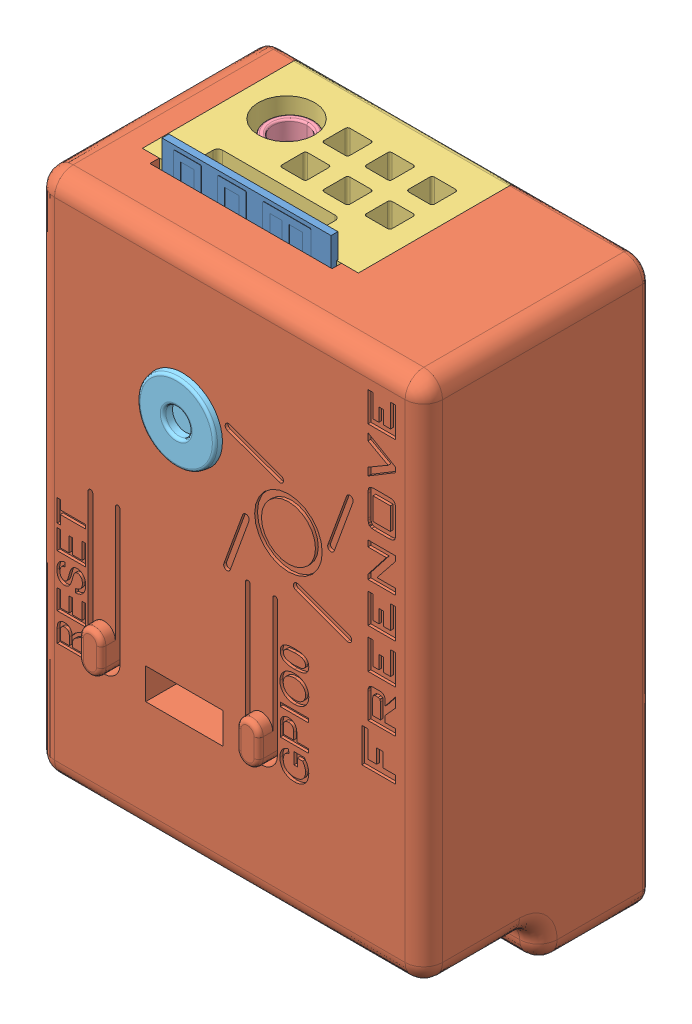
SolidWorks assembly FNK0102_Assembly_Has_Battery, configuration 默认. Lengths in mm.
Overall size (41.34 62.5 31.21).
6 component instances, 6 part files, 18 mates.
Components (placement in the parent):
- CB8201_20250427-1: CB8201_20250427 [默认] at (-3.6296 -20.6055 14.3314) x (1 0 0) z (0 0 1) size (27.94 57.2 13.09)
- FNK0102_Part1_v1.2-1: FNK0102_Part1_v1.2 [一体按键0.00间距] at (-3.8296 -20.4055 14.5) size (41.34 59.9 25.5)
- FNK0102_Part2_v1.2-1: FNK0102_Part2_v1.2 [0.0间距] at (-3.8296 30.3945 0) size (38.84 59.9 16.8)
- CB10201-1: CB10201 [默认] at (17.1633 5.4788 -53.4541) size (27.94 53.02 18.11)
- Camera_OV3660-1: Camera_OV3660 [默认] at (10.5364 16.4245 16.8) size (13.1 21.9 8.2)
- Battery_752035-1: Battery_752035 [默认] at (33.8104 2.3695 16.6198) x (0 1 0) z (-1 0 0) size (38 20 7.7)
Mates (geometry in assembly coordinates):
- 重合1: coincident: plane of assembly through (0 0 0) normal (0 0 1); plane of CB10201-1 through (-3.6296 -20.6055 0) normal (0 0 -1); plane of assembly
- 平行14: parallel: plane of assembly; plane of assembly; plane of FNK0102_Part1_v1.2-1 through (-4.0296 -20.4055 16.2) normal (1 0 0); plane of CB10201-1 through (-3.6296 30.1945 0) normal (-1 0 0)
- 重合30: coincident: plane of assembly; plane of assembly; plane of FNK0102_Part1_v1.2-1 through (-3.8296 -20.4055 -0.6) normal (0 0 -1); plane of FNK0102_Part2_v1.2-1 through (-3.8296 30.3945 -0.6) normal (0 0 1)
- 重合31: coincident: plane of assembly; plane of assembly; plane of FNK0102_Part1_v1.2-1 through (-3.8296 -26.1055 49.5331) normal (0 -1 0); plane of FNK0102_Part2_v1.2-1 through (10.1404 -26.1055 -0.6) normal (0 -1 0)
- 重合32: coincident: plane of assembly; plane of assembly; plane of FNK0102_Part1_v1.2-1 through (10.1404 -24.6055 -0.6) normal (1 0 0); plane of FNK0102_Part2_v1.2-1 through (10.1404 -24.6055 -0.6) normal (-1 0 0)
- 重合38: coincident: plane of assembly; plane of assembly; plane of CB8201_20250427-1 through (-3.6448 -20.8607 10.1) normal (0 0 -1); plane of CB10201-1 through (-1.0896 -19.3355 10.1) normal (0 0 1)
- 重合39: coincident: plane of assembly; plane of assembly; plane of CB8201_20250427-1 through (-3.4648 -20.6055 12.8952) normal (0 -1 0); plane of CB10201-1 through (-3.6296 -20.6055 10.1) normal (0 -1 0)
- 重合40: coincident: plane of assembly; plane of assembly; plane of CB8201_20250427-1 through (-3.6296 -18.2303 12.8752) normal (-1 0 0); plane of CB10201-1 through (-3.6296 -18.0655 10.1) normal (-1 0 0)
- 重合41: coincident: plane of assembly; plane of assembly; plane of FNK0102_Part1_v1.2-1 through (24.3104 -20.4055 16.2) normal (-1 0 0); plane of CB10201-1 through (24.3104 -20.6055 0) normal (1 0 0)
- 重合49: coincident: plane of assembly; plane of assembly; plane of FNK0102_Part2_v1.2-1 through (-3.8296 30.3945 0) normal (0 0 1); plane of CB10201-1 through (-3.6296 -20.6055 0) normal (0 0 -1)
- 重合50: coincident: plane of assembly; plane of assembly; plane of FNK0102_Part1_v1.2-1 through (-3.8296 -20.6055 46.3693) normal (0 -1 0); plane of CB10201-1 through (-3.6296 -20.6055 0) normal (0 -1 0)
- 同心1: concentric: cylinder of assembly; cylinder of assembly; cylinder of FNK0102_Part1_v1.2-1 through (10.1404 18.2045 21.7) axis (0 0 -1) radius 4.1; cylinder of Camera_OV3660-1 through (10.1404 18.2045 20.4) axis (0 0 -1) radius 4.1
- 平行15: parallel: plane of assembly; plane of assembly; plane of FNK0102_Part1_v1.2-1 through (-3.8296 10.4045 17.9) normal (0 1 0); plane of Camera_OV3660-1 through (13.1904 13.7545 16.9) normal (0 -1 0)
- 重合53: coincident: plane of assembly; plane of assembly; plane of FNK0102_Part1_v1.2-1 through (-3.8296 -20.4055 17.9) normal (0 0 -1); plane of Camera_OV3660-1 through (10.5364 16.4245 17.9) normal (0 0 1)
- 重合54: coincident: plane of assembly; plane of assembly; plane of FNK0102_Part1_v1.2-1 through (-3.8296 -20.4055 20.2) normal (0 0 -1); plane of Battery_752035-1 through (26.3104 -4.8055 20.2) normal (0 0 1)
- 平行16: parallel: plane of assembly; plane of assembly; plane of FNK0102_Part1_v1.2-1 through (25.8104 -22.1055 18.9) normal (1 0 0); plane of Battery_752035-1 through (26.3104 2.3695 16.6198) normal (-1 0 0)
- 距离1: distance = 0.5 mm: plane of assembly; plane of assembly; plane of Battery_752035-1 through (33.8104 2.3695 16.6198) normal (1 0 0); plane of FNK0102_Part1_v1.2-1 through (34.3104 -20.4055 -59.0874) normal (-1 0 0)
- 距离2: distance = 2 mm: plane of assembly; plane of assembly; plane of Battery_752035-1 through (26.3104 30.1945 0.2) normal (0 1 0); plane of FNK0102_Part1_v1.2-1 through (34.3104 32.1945 28.0647) normal (0 -1 0)
